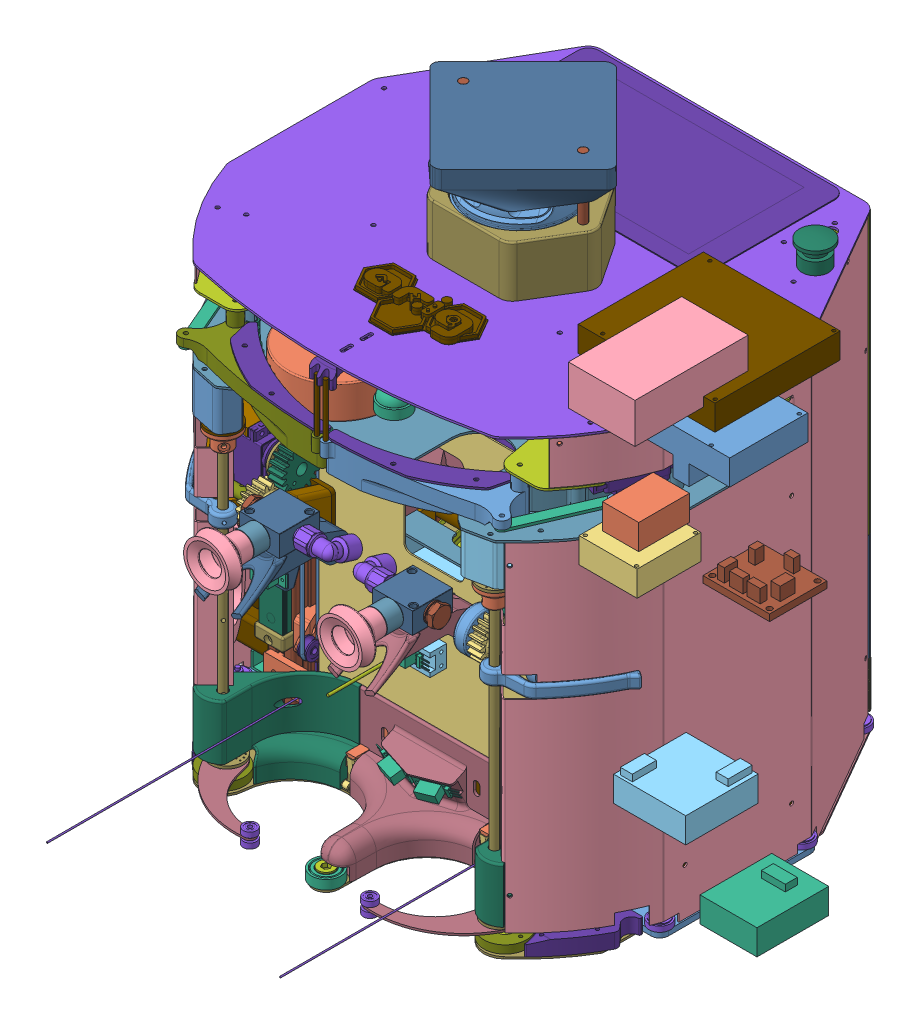
SolidWorks assembly 2019_Gros_robot, configuration Défaut. Lengths in mm.
Overall size (508.74 501.24 478.47).
582 component instances, 187 part files, 267 mates.
Components (placement in the parent):
- Robot2017_BaseRoulante-1: Robot2017_BaseRoulante [Défaut] at origin size (333 188.15 128.41)
  - Robot2015_BaseRoulante_piece01-1: Robot2015_BaseRoulante_piece01 [Défaut] at (0 7 0) size (330 4 120)
  - Robot2015_BaseRoulante_piece02-1: Robot2015_BaseRoulante_piece02 [Défaut] at (88 31 0) size (9.5 55 70)
  - Robot2015_BaseRoulante_piece02-2: Robot2015_BaseRoulante_piece02 [Défaut] at (55 31 0) x (-1 0 0) z (0 0 -1) size (9.5 55 70)
  - Robot2015_BaseRoulante_piece02-3: Robot2015_BaseRoulante_piece02 [Défaut] at (-55 31 0) size (9.5 55 70)
  - Robot2015_BaseRoulante_piece02-4: Robot2015_BaseRoulante_piece02 [Défaut] at (-88 31 0) x (-1 0 0) z (0 0 -1) size (9.5 55 70)
  - RoueMotrice-1: RoueMotrice [Défaut] at (109 -484.4772 -22.3565) x (0 -1 0) z (1 0 0) size (68.64 68.64 30)
    - Pneu-1: Pneu [Défaut] at (-515.4772 -22.3565 -15) size (64 64 30)
    - Jante-1: Jante [Défaut] at (-515.4772 -22.3565 15) x (-0.856398 -0.516316 0) z (0 0 1) size (50 50 30)
  - RoueMotrice-2: RoueMotrice [Défaut] at (-109 178.4325 494.4494) x (0 0.243951 0.969787) z (-1 0 0) size (68.64 68.64 30)
    - Pneu-1: Pneu [Défaut] at (-515.4772 -22.3565 -15) size (64 64 30)
    - Jante-1: Jante [Défaut] at (-515.4772 -22.3565 15) x (-0.856398 -0.516316 0) z (0 0 1) size (50 50 30)
  - Robot2015_BaseRoulante_piece03-1: Robot2015_BaseRoulante_piece03 [Défaut] at (117 31 0) size (67.5 12 14.69)
  - Robot2015_BaseRoulante_piece03-2: Robot2015_BaseRoulante_piece03 [Défaut] at (-117 31 0) x (-1 0 0) z (0 -0.777778 -0.62854) size (67.5 12 14.69)
  - roulement-1: roulement [Défaut] at (90 31 0) size (7 22 22)
  - roulement-2: roulement [Défaut] at (53 31 0) x (1 0 0) z (0 0.679013 0.734126) size (7 22 22)
  - roulement-3: roulement [Défaut] at (-53 31 0) x (1 0 0) z (0 0.679013 0.734126) size (7 22 22)
  - roulement-4: roulement [Défaut] at (-90 31 0) x (1 0 0) z (0 0.679013 0.734126) size (7 22 22)
  - Pignon XL037 pas5.08-1: Pignon XL037 pas5.08 [20 dents] at (67.65 31 0) x (1 0 0) z (0 -0.960015 0.27995) size (22 38 38)
  - Pignon XL037 pas5.08-2: Pignon XL037 pas5.08 [20 dents] at (67.65 149.9855 -19) x (-1 0 0) z (0 0.08811 -0.996111) size (22 38 38)
  - Robot2015_roulementAngle-1: Robot2015_roulementAngle [Défaut] at (158.5 13.75 53.5) size (16 9.5 16)
  - Robot2015_roulementAngle-2: Robot2015_roulementAngle [Défaut] at (158.5 13.75 -53.5) size (16 9.5 16)
  - Robot2015_roulementAngle-3: Robot2015_roulementAngle [Défaut] at (-158.5 13.75 53.5) size (16 9.5 16)
  - Robot2015_roulementAngle-4: Robot2015_roulementAngle [Défaut] at (-158.5 13.75 -53.5) size (16 9.5 16)
  - moteur-1: moteur [Défaut] at (48 149.9855 -19) x (0 -0.99965 -0.026437) z (1 0 0) size (42 42 188.5)
  - moteur-2: moteur [Défaut] at (-48 104.7937 -19) x (0 0.767621 0.640905) z (-1 0 0) size (42 42 188.5)
  - Pignon XL037 pas5.08-3: Pignon XL037 pas5.08 [20 dents] at (-67.65 31 0) x (-1 0 0) z (0 -0.781685 -0.623674) size (22 38 38)
  - Pignon XL037 pas5.08-4: Pignon XL037 pas5.08 [20 dents] at (-67.65 104.7937 -19) x (1 0 0) z (0 0.006752 0.999977) size (22 38 38)
  - Robot2015_profiléX20_01-1: Robot2015_profiléX20_01 [Défaut] at (-28 11 -40) x (0 0 -1) z (0 1 0) size (20 20 165)
  - Robot2015_profiléX20_01-2: Robot2015_profiléX20_01 [Défaut] at (48 11 -40) x (0 0 -1) z (0 1 0) size (20 20 165)
  - Robot2015_BaseRoulante_piece04-1: Robot2015_BaseRoulante_piece04 [Défaut] at (48 149.9855 -58) x (1 0 0) z (0 0 -1) size (3 50 44)
  - Robot2015_BaseRoulante_piece04-2: Robot2015_BaseRoulante_piece04 [Défaut] at (-51 104.7937 -58) x (1 0 0) z (0 0 -1) size (3 50 44)
  - Courroie1-5^Robot2017_BaseRoulante-1: Courroie1-5^Robot2017_BaseRoulante [Défaut] at (-67.65 104.7937 -19) x (0 0 -1) z (1 0 0) size (53.34 108.13 10) (virtual)
  - Courroie2-6^Robot2017_BaseRoulante-1: Courroie2-6^Robot2017_BaseRoulante [Défaut] at (67.65 149.9855 -19) x (0 0 1) z (-1 0 0) size (79.34 153.33 10) (virtual)
  - Robot2015_BaseRoulante_piece06-1: Robot2015_BaseRoulante_piece06 [Défaut] at (0 177.5 -61.5) size (256 20 20)
  - Igus_TK_04_09_Rail_L50-1: Igus_TK_04_09_Rail_L50 [Défaut] at (136 38.5 35) x (0 0 -1) z (1 0 0) size (9.6 50 6.3)
  - Igus_TK_04_09_coulisseau-1: Igus_TK_04_09_coulisseau [Défaut] at (136 101 35) x (0 0 -1) z (1 0 0) size (20 29 8.3)
  - Igus_TK_04_09_Rail_L50-2: Igus_TK_04_09_Rail_L50 [Défaut] at (136 38.5 -35) x (0 0 -1) z (1 0 0) size (9.6 50 6.3)
  - Igus_TK_04_09_coulisseau-2: Igus_TK_04_09_coulisseau [Défaut] at (136 101 -35) x (0 0 -1) z (1 0 0) size (20 29 8.3)
  - Igus_TK_04_09_Rail_L50-3: Igus_TK_04_09_Rail_L50 [Défaut] at (-136 38.5 35) x (0 0 1) z (-1 0 0) size (9.6 50 6.3)
  - Igus_TK_04_09_coulisseau-3: Igus_TK_04_09_coulisseau [Défaut] at (-136 101 35) x (0 0 1) z (-1 0 0) size (20 29 8.3)
  - Igus_TK_04_09_Rail_L50-4: Igus_TK_04_09_Rail_L50 [Défaut] at (-136 38.5 -35) x (0 0 1) z (-1 0 0) size (9.6 50 6.3)
  - Igus_TK_04_09_coulisseau-4: Igus_TK_04_09_coulisseau [Défaut] at (-136 101 -35) x (0 0 1) z (-1 0 0) size (20 29 8.3)
  - Kubler-05.2400.1212.1024-1: Kubler-05.2400.1212.1024 [fil a Gch] at (157 24 0) x (-1 0 0) z (0 0.34202 0.939693) size (31 88.25 62)
    - Kubler-05.2400.1212.1024-1: Kubler-05.2400.1212.1024 [Défaut] at origin size (31 36 24)
    - Kubler-rayon mini cable-1: Kubler-rayon mini cable [Défaut] at (25 -24 0) x (0 0 1) z (-1 0 0) size (52.25 52.25 4.5)
  - Kubler-05.2400.1212.1024-2: Kubler-05.2400.1212.1024 [fil a Drt] at (-157 24 0) x (1 0 0) z (0 -0.34202 -0.939693) size (31 88.25 62)
    - Kubler-05.2400.1212.1024-1: Kubler-05.2400.1212.1024 [Défaut] at origin size (31 36 24)
    - Kubler-rayon mini cable-1: Kubler-rayon mini cable [Défaut] at (25 -24 0) x (0 0 -1) z (1 0 0) size (52.25 52.25 4.5)
  - Robot2015_BaseRoulante_piece07-1: Robot2015_BaseRoulante_piece07 [Défaut] at (146 56.5 0) x (0 0 -1) z (1 0 0) size (93 50 1.5)
  - Robot2015_BaseRoulante_piece07-2: Robot2015_BaseRoulante_piece07 [Défaut] at (-146 56.5 0) x (0 0 1) z (-1 0 0) size (93 50 1.5)
  - Robot2015_BaseRoulante_piece08-1: Robot2015_BaseRoulante_piece08 [Défaut] at (51 38.5 30) size (85 55 10)
  - Robot2015_BaseRoulante_piece09-1: Robot2015_BaseRoulante_piece09 [Défaut] at (51 38.5 -30) x (1 0 0) z (0 0 -1) size (57 55 10)
  - Robot2015_BaseRoulante_piece09-2: Robot2015_BaseRoulante_piece09 [Défaut] at (-51 38.5 -30) x (-1 0 0) z (0 0 -1) size (57 55 10)
  - Robot2015_BaseRoulante_piece08-2: Robot2015_BaseRoulante_piece08 [Défaut] at (-51 38.5 30) x (-1 0 0) z (0 0 1) size (85 55 10)
  - Robot2015_BaseRoulante_piece10-1: Robot2015_BaseRoulante_piece10 [Défaut] at (155 24 0) x (-1 0 0) z (0 -0.545932 -0.837829) size (9 48 48)
  - Robot2015_BaseRoulante_piece10-2: Robot2015_BaseRoulante_piece10 [Défaut] at (-155 24 0) size (9 48 48)
  - Robot2015_BaseRoulante_piece11-1: Robot2015_BaseRoulante_piece11 [Défaut] at (79 66 0) x (0 0 -1) z (1 0 0) size (80 1.5 63)
  - Robot2015_BaseRoulante_piece11-2: Robot2015_BaseRoulante_piece11 [Défaut] at (-79 66 0) x (0 0 1) z (-1 0 0) size (80 1.5 63)
  - Robot2015_BaseRoulante_piece12-1: Robot2015_BaseRoulante_piece12 [Défaut] at (162 11 40) x (-1 0 0) z (0 0 -1) size (11.5 11.5 80)
  - Robot2015_BaseRoulante_piece12-2: Robot2015_BaseRoulante_piece12 [Défaut] at (-162 11 -40) size (11.5 11.5 80)
  - pignon renvoi 20 dents XL 2006-1: pignon renvoi 20 dents XL 2006 [Défaut] at (67.65 40 -45) x (1 0 0) z (0 0.474564 0.880221) size (9 32.34 32.34)
  - 20170402-1131-1: 20170402-1131 [Défaut] at (48 40 -45) x (0 0 -1) z (1 0 0) size (25 50 24.65)
  - 20170402-1229-1: 20170402-1229 [Défaut] at (73.15 40 -38.5) x (0 0 -1) z (1 0 0) size (25.5 30 9)
- batterieLIPO-1: batterieLIPO [Défaut] at (-65 97 -76) size (160 49 34)
- Robot2019_profiléX20_02-1: Robot2019_profiléX20_02 [Défaut] at (-110 276 40) x (0 0 1) z (0 -1 0) size (20 20 265)
- Robot2019_profiléX20_02-2: Robot2019_profiléX20_02 [Défaut] at (-110 276 -60) x (0 0 1) z (0 -1 0) size (20 20 265)
- Robot2019_profiléX20_02-3: Robot2019_profiléX20_02 [Défaut] at (130 276 40) x (0 0 1) z (0 -1 0) size (20 20 265)
- Robot2019_profiléX20_02-4: Robot2019_profiléX20_02 [Défaut] at (130 276 -60) x (0 0 1) z (0 -1 0) size (20 20 265)
- Robot2019_plaque bille porteuseAvant-1: Robot2019_plaque bille porteuseAvant [Défaut] at (0 5.5 0) size (300 1.5 120)
- Robot2019_plaque bille porteuse Arriere-1: Robot2019_plaque bille porteuse Arriere [Défaut] at (0 5.5 0) x (-1 0 0) z (0 0 -1) size (310 1.5 125)
- Robot2019_plaque du dessus-1: Robot2019_plaque du dessus [Défaut] at (0 276 0) size (330 1.5 300.96)
- APEM_A01ES_A0154B-1: APEM_A01ES_A0154B [Défaut] at (121.8383 345 -100) x (0.5 0 0.866025) z (-0.866025 0 0.5) size (24 61 24)
- bille porteuse-3: bille porteuse [Défaut] at (-111.446 0 -110) x (-0.5 0 -0.866025) z (0.866025 0 -0.5) size (49.64 21.5 47.15)
  - Robot2015_support bille porteuse-1: Robot2015_support bille porteuse [Défaut] at (0 9.5 0) size (49.64 12 45)
  - BillePorteuse-1: BillePorteuse [Défaut] at (0 7.5 0) x (0.947171 0 0.32073) z (0.32073 0 -0.947171) size (31 21.5 31)
- bille porteuse-4: bille porteuse [Défaut] at (111.446 0 -110) size (49.64 21.5 47.15)
  - Robot2015_support bille porteuse-1: Robot2015_support bille porteuse [Défaut] at (0 9.5 0) size (49.64 12 45)
  - BillePorteuse-1: BillePorteuse [Défaut] at (0 7.5 0) x (0.947171 0 0.32073) z (0.32073 0 -0.947171) size (31 21.5 31)
- pompe air 12v SFE-1: pompe air 12v SFE [Défaut] at (-20.6394 32 -38) size (38 60 92)
- rplidar-a2-1: rplidar-a2 [Défaut] at (-75 354.2861 -6.0269) x (0 0 -1) z (1 0 0) size (80.61 40.81 84.84)
- Robot2015_roulementAngle-1: Robot2015_roulementAngle [Défaut] at (100.765 9.75 -153.5) size (16 9.5 16)
- Robot2015_roulementAngle-2: Robot2015_roulementAngle [Défaut] at (-100.765 9.75 -153.5) size (16 9.5 16)
- 20180929-0119-1: 20180929-0119 [Défaut] at (0 277.5 0) x (-1 0 0) z (0 0 -1) size (291.8 157.5 260.35) (flexible)
  - Palet-1: Palet [Redium] at (-99.9974 12.7 0.7186) size (76.2 25.4 76.2)
  - Palet-2: Palet [Greenium] at (-49.3764 12.7 86.9596) size (76.2 25.4 76.2)
  - Palet-3: Palet [Redium] at (50.6211 12.7 86.241) size (76.2 25.4 76.2) (hidden)
  - Palet-4: Palet [Blueium] at (99.9974 12.7 -0.7186) x (0.648467 0 0.761243) z (-0.761243 0 0.648467) size (76.2 25.4 76.2)
  - Palet-5: Palet [Greenium] at (49.3764 12.7 -86.9596) x (0.321702 0 0.946841) z (-0.946841 0 0.321702) size (76.2 25.4 76.2)
  - Palet-6: Palet [Redium] at (-50.6211 12.7 -86.241) size (76.2 25.4 76.2) (hidden)
  - roulement-1: roulement [Défaut] at (81.9289 14.5 -48.09) x (0 -1 0) z (0.925744 0 -0.37815) size (7 22 22)
  - roulement-2: roulement [Défaut] at (-0.6827 14.5 -94.9975) x (0 -1 0) z (0.135385 0 -0.990793) size (7 22 22)
  - roulement-3: roulement [Défaut] at (-82.6116 14.5 -46.9075) x (0 -1 0) z (-0.79036 0 -0.612643) size (7 22 22)
  - roulement-4: roulement [Défaut] at (-81.9289 14.5 48.09) x (0 -1 0) z (-0.925744 0 0.37815) size (7 22 22)
  - roulement-5: roulement [Défaut] at (0.6827 14.5 94.9975) x (0 -1 0) z (-0.135385 0 0.990793) size (7 22 22)
  - roulement-6: roulement [Défaut] at (82.6116 14.5 46.9075) x (0 -1 0) z (0.79036 0 0.612643) size (7 22 22)
  - 20181010-0238-1: 20181010-0238 [Défaut] at (0 8.5 -22.5) x (0.926307 0 0.37677) z (-0.37677 0 0.926307) size (29.93 18 29.98)
  - 20181010-0239-1: 20181010-0239 [Défaut] at (0 8.5 0) x (0.853252 0 -0.521498) z (0.521498 0 0.853252) size (122.02 20.9 126.29)
  - PlaqueTounanteCarre94mm-1: PlaqueTounanteCarre94mm [Défaut] x (-0.707107 0 0.707107) z (-0.707107 0 -0.707107) size (115.6 8.5 115.6) (flexible)
    - PlaqueTounanteCarre94mm-1: PlaqueTounanteCarre94mm [Défaut] at origin size (94 8.25 94)
    - PlaqueTounanteCarre94mm-2: PlaqueTounanteCarre94mm [Défaut] at (0 8.5 0) x (-0.265754 0 -0.964041) z (-0.964041 0 0.265754) size (94 8.25 94)
  - 20190123-2151-1: 20190123-2151 [Défaut] at (0 16.5 0) x (-0.506211 0 -0.86241) z (0.86241 0 -0.506211) size (41.57 20.66 45)
  - 20190123-2208-1: 20190123-2208 [Défaut] at (81.9289 17.9 -48.09) x (-0.274765 0 -0.961511) z (-0.961511 0 0.274765) size (11.85 7.9 11.85)
  - 20190123-2208-2: 20190123-2208 [Défaut] at (-0.6827 17.9 -94.9975) x (-0.970076 0 -0.242802) z (-0.242802 0 0.970076) size (11.85 7.9 11.85)
  - 20190123-2208-3: 20190123-2208 [Défaut] at (-82.6116 17.9 -46.9075) x (-0.695311 0 0.718709) z (0.718709 0 0.695311) size (11.85 7.9 11.85)
  - 20190123-2208-4: 20190123-2208 [Défaut] at (-81.9289 17.9 48.09) x (0.274765 0 0.961511) z (0.961511 0 -0.274765) size (11.85 7.9 11.85)
  - 20190123-2208-5: 20190123-2208 [Défaut] at (0.6827 17.9 94.9975) x (0.970076 0 0.242802) z (0.242802 0 -0.970076) size (11.85 7.9 11.85)
  - 20190123-2208-6: 20190123-2208 [Défaut] at (82.6116 17.9 46.9075) x (0.695311 0 -0.718709) z (-0.718709 0 -0.695311) size (11.85 7.9 11.85)
  - 20190123-2151-2: 20190123-2151 [Défaut] at (0 16.5 0) x (-0.999974 0 0.007186) z (-0.007186 0 -0.999974) size (41.57 20.66 45)
  - 20190123-2151-3: 20190123-2151 [Défaut] at (0 16.5 0) x (-0.493764 0 0.869596) z (-0.869596 0 -0.493764) size (41.57 20.66 45)
  - 20190123-2151-4: 20190123-2151 [Défaut] at (0 16.5 0) x (0.506211 0 0.86241) z (-0.86241 0 0.506211) size (41.57 20.66 45)
  - 20190123-2151-5: 20190123-2151 [Défaut] at (0 16.5 0) x (0.999974 0 -0.007186) z (0.007186 0 0.999974) size (41.57 20.66 45)
  - 20190123-2151-6: 20190123-2151 [Défaut] at (0 16.5 0) x (0.493764 0 -0.869596) z (0.869596 0 0.493764) size (41.57 20.66 45)
  - 12v-silent-dc-motor-146rpm-encoder-desc-dime-1: 12v-silent-dc-motor-146rpm-encoder-desc-dime [Défaut] at (0 -2.5 -22.5) x (0 -1 0) z (-0.707107 0 -0.707107) size (123 36 36)
  - 20190124-0048-1: 20190124-0048 [Défaut] at (0 26.5 -22.5) size (15 43 15)
  - NBB1,5-F79-E0-1: NBB1,5-F79-E0 [Défaut] at (43 30 0) x (1 0 0) z (0 0 -1) size (21 4.7 8)
  - 20190124-0123-1: 20190124-0123 [Défaut] at (47 32 -6.05) x (0 0 1) z (-1 0 0) size (19 4 16)
- 20181001-1750-1: 20181001-1750 [Défaut] at origin size (319.23 219.5 239.4)
  - Access_HS-645_BrasRondPetitModele-2: Access_HS-645_BrasRondPetitModele [Défaut] at (94 204.5566 85.221) x (0 0.153259 -0.988186) z (0 0.988186 0.153259) size (24 5 24)
  - Palet-1: Palet [Redium] at (50 201.2365 189.2) x (1 0 0) z (0 1 0) size (76.2 25.4 76.2) (hidden)
  - Servo_HS-805-BB-1: Servo_HS-805-BB [Défaut] at (-29 228 9) x (0 0.965926 -0.258819) z (0 0.258819 0.965926) size (82 65 29.5)
  - Access_HS-805_BrasRond-1: Access_HS-805_BrasRond [Défaut] at (-89 228 9) x (0 0 -1) z (0 1 0) size (39.6 8.5 39.6)
  - HIWIN_MGW09H 1 R 200 ZF H M SS_FILE-1: HIWIN_MGW09H 1 R 200 ZF H M SS_FILE [Défaut] at (-120 68 60) size (18 200 7)
  - HIWIN_MGW09H 1 R 200 ZF H M SS_FILE_1-1: HIWIN_MGW09H 1 R 200 ZF H M SS_FILE_1 [Défaut] at (-120 164.4365 60) size (30 51.3 9.1)
  - HIWIN_MGW09H 1 R 200 ZF H M SS_FILE-2: HIWIN_MGW09H 1 R 200 ZF H M SS_FILE [Défaut] at (120 68 60) size (18 200 7)
  - HIWIN_MGW09H 1 R 200 ZF H M SS_FILE_1-2: HIWIN_MGW09H 1 R 200 ZF H M SS_FILE_1 [Défaut] at (120 164.4365 60) size (30 51.3 9.1)
  - Galet_RainureU_4x13x7-1: Galet_RainureU_4x13x7 [Défaut] at (-95.5 68 62) x (1 0 0) z (0 1 0) size (7 13 13)
  - Galet_RainureU_4x13x7-2: Galet_RainureU_4x13x7 [Défaut] at (-95.5 188 50) x (1 0 0) z (0 1 0) size (7 13 13)
  - 20190123-2357-1: 20190123-2357 [Défaut] at (-98 228 9) x (1 0 0) z (0 0 -1) size (7 93 93)
  - Galet_RainureU_4x13x7-5: Galet_RainureU_4x13x7 [Défaut] at (-95.5 248 62) x (1 0 0) z (0 1 0) size (7 13 13)
  - 20190124-0203-1: 20190124-0203 [Défaut] at (-95.5 68 68) x (0 0 1) z (-1 0 0) size (104.52 211.5 2.55)
  - Servo_HS-805-BB-3: Servo_HS-805-BB [Défaut] at (29 228 9) x (0 0.965926 -0.258819) z (0 -0.258819 -0.965926) size (82 65 29.5)
  - SymétrieAccess_HS-805_BrasRond-3: SymétrieAccess_HS-805_BrasRond [Défaut] at (89 228 9) x (0 0 -1) z (0 -1 0) size (39.6 8.5 39.6)
  - 20190123-2357-3: 20190123-2357 [Défaut] at (98 228 9) x (-1 0 0) z (0 0 1) size (7 93 93)
  - Symétrie20190124-0203-2: Symétrie20190124-0203 [Défaut] at (95.5 68 68) x (0 0 1) z (-1 0 0) size (104.5 211.5 2.5)
  - Galet_RainureU_4x13x7-7: Galet_RainureU_4x13x7 [Défaut] at (95.5 248 62) x (-1 0 0) z (0 -1 0) size (7 13 13)
  - Galet_RainureU_4x13x7-8: Galet_RainureU_4x13x7 [Défaut] at (95.5 188 50) x (-1 0 0) z (0 -1 0) size (7 13 13)
  - Galet_RainureU_4x13x7-9: Galet_RainureU_4x13x7 [Défaut] at (95.5 68 62) x (-1 0 0) z (0 -1 0) size (7 13 13)
  - Ventouse_D33-1: Ventouse_D33 [Défaut] at (50 206.2365 176.5) x (1 0 0) z (0 1 0) size (36.31 27 36.31)
  - 20170416-2304-1: 20170416-2304 [Défaut] at (54 176.4365 124) size (30.6 16 70.4)
    - SupportCapteurPololu-1: SupportCapteurPololu [Défaut] at origin size (30 16 12.5) (hidden)
    - pololu gp2y0d805-1: pololu gp2y0d805 [Défaut] at (-14.5 -4.5 10.8) size (30.1 9 11.8)
    - faisceau pololu gp2y0d-1: faisceau pololu gp2y0d [5cm] at (-3.9 0 20.4) size (2 2 50) (hidden)
  - Legris_EQUERRE-OSCILLANTE_3159_06_10-1: Legris_EQUERRE-OSCILLANTE_3159_06_10 [Défaut] at (40 206.2365 130.5) x (0 -0.296934 -0.954898) z (0 0.954898 -0.296934) size (28 34.3 15.01)
  - Legris_DouilleAnnelee_0934_10_10-1: Legris_DouilleAnnelee_0934_10_10 [Défaut] at (50 206.2365 151) x (-0.990503 0.137493 0) z (0.137493 0.990503 0) size (15.24 32.5 12)
  - Legris_NourriceCroix_3312_00_10-1: Legris_NourriceCroix_3312_00_10 [Défaut] at (50 198.2365 130.5) x (1 0 0) z (0 1 0) size (30 30 16)
  - Legris_Bouchon_0220_10_00-1: Legris_Bouchon_0220_10_00 [Défaut] at (67.975 206.2365 130.5) x (-1 0 0) z (0 -1 0) size (12.5 14 16.17)
  - 20181010-0238-2: 20181010-0238 [Défaut] at (78 184.2365 103) x (0 0.752597 -0.658481) z (0 -0.658481 -0.752597) size (29.93 18 29.98)
  - roulement_D8-D16-ep4-2: roulement_D8-D16-ep4 [Défaut] at (121.5 184.2365 103) x (1 0 0) z (0 -0.7977 0.603055) size (4 16 16)
  - 20190206-2329-1: 20190206-2329 [Défaut] at (50 206.2365 176.5) size (36.88 28.38 83.9)
  - 20190207-0044-1: 20190207-0044 [Défaut] at (50 206.2365 158.5) x (0.792778 -0.60951 0) z (0 0 -1) size (18 18 13)
  - 20181010-0240-1: 20181010-0240 [Défaut] at (78.5 204.5566 85.221) x (0 0.752597 -0.658481) z (0 -0.658481 -0.752597) size (29.93 11 29.98)
  - 20190207-0111-1: 20190207-0111 [Défaut] at (33.5 184.2365 103) x (0 -0.34202 -0.939693) z (-1 0 0) size (8 8 90)
  - roulement-1: roulement [Défaut] at (70 184.2365 103) size (7 22 22)
  - Servo_HS-645-MG_2-1: Servo_HS-645-MG_2 [Défaut] at (134.238 174.3306 75.442) x (0 0 1) z (0 -1 0) size (19.56 43.24 53.34)
  - 20190208-1431-1: 20190208-1431 [Défaut] at (66.5 164.2365 72) size (75 57 3)
  - 20190208-1506-1: 20190208-1506 [Défaut] at (109 221.2365 75) x (1 0 0) z (0 -1 0) size (76.02 43 57.11)
  - 20190209-0034-1: 20190209-0034 [Défaut] at (-110 68 50) x (0 0 1) z (1 0 0) size (24.5 25 12.5)
  - 20190209-0034-2: 20190209-0034 [Défaut] at (-110 248 50) x (0 0 1) z (1 0 0) size (24.5 25 12.5)
  - 20190209-0206-1: 20190209-0206 [Défaut] at (-110 200.5 50) x (0 0 -1) z (1 0 0) size (16 25 12.5)
  - 20190209-0206-2: 20190209-0206 [Défaut] at (110 200.5 50) x (0 0 1) z (-1 0 0) size (16 25 12.5)
  - 20190209-0034-3: 20190209-0034 [Défaut] at (110 248 50) x (0 0 1) z (-1 0 0) size (24.5 25 12.5)
  - 20190209-0034-4: 20190209-0034 [Défaut] at (110 68 50) x (0 0 1) z (-1 0 0) size (24.5 25 12.5)
  - 20190211-2116-1: 20190211-2116 [Défaut] at (148.047 126.5 67.5372) x (0.819152 0 0.573576) z (-0.573576 0 0.819152) size (12 78.68 50)
  - Igus_ChainePorteCable_ExtremiteA_modif2019-1: Igus_ChainePorteCable_ExtremiteA_modif2019 [Défaut] at (150.9141 126.5 69.5447) x (0 1 0) z (-0.573576 0 0.819152) size (26 36.15 16.39)
  - Igus_ChainePorteCable_ExtremiteB_modif2019-1: Igus_ChainePorteCable_ExtremiteB_modif2019 [Défaut] at (155.7489 239.4042 62.6133) x (0.099601 0.984808 -0.142244) z (-0.564863 0.173648 0.806707) size (25.74 12 18.61)
  - 20190212-2242-1: 20190212-2242 [Défaut] at (93.5 179.2365 72) size (8 24 3.9)
  - 20190212-2242-2: 20190212-2242 [Défaut] at (93.5 179.2365 64.2) x (1 0 0) z (0 0 -1) size (8 24 3.9)
  - 20190328-0013-1: 20190328-0013 [Défaut] at (73.5 184.2365 103) x (0 -0.835831 -0.548987) z (0 -0.548987 0.835831) size (14 4.5 14)
  - 20190208-1431-2: 20190208-1431 [Défaut] at (-66.5 164.2365 75) x (-1 0 0) z (0 0 -1) size (75 57 3)
  - Symétrie20190208-1506-2: Symétrie20190208-1506 [Défaut] at (-109 221.2365 75) x (-1 0 0) z (0 1 0) size (76.02 43 57.11)
  - Servo_HS-645-MG_2-2: Servo_HS-645-MG_2 [Défaut] at (-134.238 174.3306 95) x (0 0 -1) z (0 -1 0) size (19.56 43.24 53.34)
  - Access_HS-645_BrasRondPetitModele-3: Access_HS-645_BrasRondPetitModele [Défaut] at (-89 204.5566 85.221) x (0 -0.153259 0.988186) z (0 -0.988186 -0.153259) size (24 5 24)
  - 20181010-0240-2: 20181010-0240 [Défaut] at (-89.5 204.5566 85.221) x (0 0.752597 -0.658481) z (0 -0.658481 -0.752597) size (29.93 11 29.98)
  - 20181010-0238-3: 20181010-0238 [Défaut] at (-96 184.2365 103) x (0 0.752597 -0.658481) z (0 -0.658481 -0.752597) size (29.93 18 29.98)
  - 20190328-0013-2: 20190328-0013 [Défaut] at (-73.5 184.2365 103) x (0 -0.835831 -0.548987) z (0 0.548987 -0.835831) size (14 4.5 14)
  - 20190207-0111-2: 20190207-0111 [Défaut] at (-123.5 184.2365 103) x (0 -0.34202 -0.939693) z (-1 0 0) size (8 8 90)
  - Symétrie20190206-2329-2: Symétrie20190206-2329 [Défaut] at (-50 206.2365 176.5) x (-1 0 0) z (0 0 -1) size (36.88 28.38 83.9)
  - roulement_D8-D16-ep4-3: roulement_D8-D16-ep4 [Défaut] at (-121.5 184.2365 103) x (-1 0 0) z (0 0.7977 -0.603055) size (4 16 16)
  - roulement-2: roulement [Défaut] at (-70 184.2365 103) x (-1 0 0) z (0 0 -1) size (7 22 22)
  - 20170416-2304-2: 20170416-2304 [Défaut] at (-54 176.4365 124) x (-1 0 0) z (0 0 1) size (30.6 16 70.4)
    - SupportCapteurPololu-1: SupportCapteurPololu [Défaut] at origin size (30 16 12.5) (hidden)
    - pololu gp2y0d805-1: pololu gp2y0d805 [Défaut] at (-14.5 -4.5 10.8) size (30.1 9 11.8)
    - faisceau pololu gp2y0d-1: faisceau pololu gp2y0d [5cm] at (-3.9 0 20.4) size (2 2 50) (hidden)
  - Legris_NourriceCroix_3312_00_10-2: Legris_NourriceCroix_3312_00_10 [Défaut] at (-50 214.2365 130.5) x (-1 0 0) z (0 -1 0) size (30 30 16)
  - Legris_Bouchon_0220_10_00-2: Legris_Bouchon_0220_10_00 [Défaut] at (-67.975 206.2365 130.5) x (1 0 0) z (0 1 0) size (12.5 14 16.17)
  - SymétrieIgus_ChainePorteCable_ExtremiteA_modif2019-2: SymétrieIgus_ChainePorteCable_ExtremiteA_modif2019 [Défaut] at (-150.9141 126.5 69.5447) x (0 1 0) z (-0.573576 0 -0.819152) size (26 36.15 16.39)
  - 20190211-2116-2: 20190211-2116 [Défaut] at (-148.047 126.5 67.5372) x (0.819152 0 -0.573576) z (0.573576 0 0.819152) size (12 78.68 50)
  - Igus_ChainePorteCable_ExtremiteB_modif2019-2: Igus_ChainePorteCable_ExtremiteB_modif2019 [Défaut] at (-150.0148 239.4042 58.5983) x (-0.099601 0.984808 -0.142244) z (0.564863 0.173648 0.806707) size (25.74 12 18.61)
  - 20190207-0044-2: 20190207-0044 [Défaut] at (-50 206.2365 158.5) x (0.792778 0.60951 0) z (0 0 -1) size (18 18 13)
  - Ventouse_D33-2: Ventouse_D33 [Défaut] at (-50 206.2365 176.5) x (-1 0 0) z (0 -1 0) size (36.31 27 36.31)
  - Legris_DouilleAnnelee_0934_10_10-2: Legris_DouilleAnnelee_0934_10_10 [Défaut] at (-50 206.2365 151) x (0.990503 0.137493 0) z (0.137493 -0.990503 0) size (15.24 32.5 12)
  - Legris_EQUERRE-OSCILLANTE_3159_06_10-2: Legris_EQUERRE-OSCILLANTE_3159_06_10 [Défaut] at (-40 206.2365 130.5) x (0 -0.296934 -0.954898) z (0 -0.954898 0.296934) size (28 34.3 15.01)
  - 20190409-2355-1: 20190409-2355 [Défaut] at (120 61 60) size (22 10 10.2)
  - 20190409-2355-2: 20190409-2355 [Défaut] at (120 275 60) x (-1 0 0) z (0 0 1) size (22 10 10.2)
  - 20190409-2355-3: 20190409-2355 [Défaut] at (-120 275 60) x (-1 0 0) z (0 0 1) size (22 10 10.2)
  - 20190409-2355-4: 20190409-2355 [Défaut] at (-120 61 60) size (22 10 10.2)
- 20181001-2148-1: 20181001-2148 [Défaut] at (-50 7 120) size (106 62 83)
- 20181002-0030-1: 20181002-0030 [Défaut] at (0 277.5 0) x (0.725374 0 0.688355) z (-0.688355 0 0.725374) size (312.09 32 306.03)
  - 20181002-0031-1: 20181002-0031 [Défaut] at origin size (146.08 16 151.84)
  - BagueRivetAIRBUS-1: BagueRivetAIRBUS [Défaut] at (141.5 15.8 0) x (0.352131 0 0.935951) z (0 1 0) size (6.8 6.8 5.6)
  - BagueRivetAIRBUS-2: BagueRivetAIRBUS [Défaut] at (141.3061 15.8 -7.4055) x (0.400633 0 0.916239) z (0 1 0) size (6.8 6.8 5.6)
  - BagueRivetAIRBUS-3: BagueRivetAIRBUS [Défaut] at (140.7248 15.8 -14.7908) x (0.448036 0 0.894016) z (0 1 0) size (6.8 6.8 5.6)
  - BagueRivetAIRBUS-4: BagueRivetAIRBUS [Défaut] at (139.7579 15.8 -22.1355) x (0.494211 0 0.869342) z (0 1 0) size (6.8 6.8 5.6)
  - BagueRivetAIRBUS-5: BagueRivetAIRBUS [Défaut] at (138.4079 15.8 -29.4195) x (0.539032 0 0.842286) z (0 1 0) size (6.8 6.8 5.6)
  - BagueRivetAIRBUS-6: BagueRivetAIRBUS [Défaut] at (136.6785 15.8 -36.6229) x (0.582375 0 0.812921) z (0 1 0) size (6.8 6.8 5.6)
  - BagueRivetAIRBUS-7: BagueRivetAIRBUS [Défaut] at (134.5745 15.8 -43.7259) x (0.624122 0 0.781327) z (0 1 0) size (6.8 6.8 5.6)
  - BagueRivetAIRBUS-8: BagueRivetAIRBUS [Défaut] at (132.1016 15.8 -50.7091) x (0.664158 0 0.747593) z (0 1 0) size (6.8 6.8 5.6)
  - BagueRivetAIRBUS-9: BagueRivetAIRBUS [Défaut] at (129.2667 15.8 -57.5532) x (0.702373 0 0.711809) z (0 1 0) size (6.8 6.8 5.6)
  - BagueRivetAIRBUS-10: BagueRivetAIRBUS [Défaut] at (126.0774 15.8 -64.2397) x (0.738664 0 0.674074) z (0 1 0) size (6.8 6.8 5.6)
  - BagueRivetAIRBUS-11: BagueRivetAIRBUS [Défaut] at (122.5426 15.8 -70.75) x (0.77293 0 0.634491) z (0 1 0) size (6.8 6.8 5.6)
  - BagueRivetAIRBUS-12: BagueRivetAIRBUS [Défaut] at (118.6719 15.8 -77.0664) x (0.805077 0 0.59317) z (0 1 0) size (6.8 6.8 5.6)
  - BagueRivetAIRBUS-13: BagueRivetAIRBUS [Défaut] at (114.4759 15.8 -83.1716) x (0.835018 0 0.550222) z (0 1 0) size (6.8 6.8 5.6)
  - BagueRivetAIRBUS-14: BagueRivetAIRBUS [Défaut] at (109.9662 15.8 -89.0488) x (0.86267 0 0.505767) z (0 1 0) size (6.8 6.8 5.6)
  - BagueRivetAIRBUS-15: BagueRivetAIRBUS [Défaut] at (105.155 15.8 -94.682) x (0.887958 0 0.459925) z (0 1 0) size (6.8 6.8 5.6)
  - BagueRivetAIRBUS-16: BagueRivetAIRBUS [Défaut] at (100.0556 15.8 -100.0556) x (0.910812 0 0.412822) z (0 1 0) size (6.8 6.8 5.6)
  - BagueRivetAIRBUS-17: BagueRivetAIRBUS [Défaut] at (94.682 15.8 -105.155) x (0.931169 0 0.364589) z (0 1 0) size (6.8 6.8 5.6)
  - BagueRivetAIRBUS-18: BagueRivetAIRBUS [Défaut] at (89.0488 15.8 -109.9662) x (0.948974 0 0.315355) z (0 1 0) size (6.8 6.8 5.6)
  - BagueRivetAIRBUS-19: BagueRivetAIRBUS [Défaut] at (83.1716 15.8 -114.4759) x (0.964178 0 0.265258) z (0 1 0) size (6.8 6.8 5.6)
  - BagueRivetAIRBUS-20: BagueRivetAIRBUS [Défaut] at (77.0664 15.8 -118.6719) x (0.976739 0 0.214433) z (0 1 0) size (6.8 6.8 5.6)
  - BagueRivetAIRBUS-21: BagueRivetAIRBUS [Défaut] at (70.75 15.8 -122.5426) x (0.986623 0 0.163021) z (0 1 0) size (6.8 6.8 5.6)
  - BagueRivetAIRBUS-22: BagueRivetAIRBUS [Défaut] at (64.2397 15.8 -126.0774) x (0.993802 0 0.111161) z (0 1 0) size (6.8 6.8 5.6)
  - BagueRivetAIRBUS-23: BagueRivetAIRBUS [Défaut] at (57.5532 15.8 -129.2667) x (0.998258 0 0.058997) z (0 1 0) size (6.8 6.8 5.6)
  - BagueRivetAIRBUS-24: BagueRivetAIRBUS [Défaut] at (50.7091 15.8 -132.1016) x (0.999978 0 0.006672) z (0 1 0) size (6.8 6.8 5.6)
  - BagueRivetAIRBUS-25: BagueRivetAIRBUS [Défaut] at (43.7259 15.8 -134.5745) x (0.998956 0 -0.045672) z (0 1 0) size (6.8 6.8 5.6)
  - BagueRivetAIRBUS-26: BagueRivetAIRBUS [Défaut] at (36.6229 15.8 -136.6785) x (0.995197 0 -0.097891) z (0 1 0) size (6.8 6.8 5.6)
  - BagueRivetAIRBUS-27: BagueRivetAIRBUS [Défaut] at (29.4195 15.8 -138.4079) x (0.98871 0 -0.149841) z (0 1 0) size (6.8 6.8 5.6)
  - BagueRivetAIRBUS-28: BagueRivetAIRBUS [Défaut] at (22.1355 15.8 -139.7579) x (0.979513 0 -0.201381) z (0 1 0) size (6.8 6.8 5.6)
  - BagueRivetAIRBUS-29: BagueRivetAIRBUS [Défaut] at (14.7908 15.8 -140.7248) x (0.967631 0 -0.252369) z (0 1 0) size (6.8 6.8 5.6)
  - BagueRivetAIRBUS-30: BagueRivetAIRBUS [Défaut] at (7.4055 15.8 -141.3061) x (0.953097 0 -0.302665) z (0 1 0) size (6.8 6.8 5.6)
  - 20181002-0031-2: 20181002-0031 [Défaut] at (0 32 0) x (0.052336 0 -0.99863) z (-0.99863 0 -0.052336) size (146.08 16 151.84)
  - 20181002-0031-3: 20181002-0031 [Défaut] x (0 0 -1) z (1 0 0) size (146.08 16 151.84)
  - 20181002-0031-4: 20181002-0031 [Défaut] x (-1 0 0) z (0 0 -1) size (146.08 16 151.84)
  - BagueRivetAIRBUS-91: BagueRivetAIRBUS [Défaut] at (0 15.8 -141.5) x (0.935951 0 -0.352131) z (0 1 0) size (6.8 6.8 5.6)
  - BagueRivetAIRBUS-92: BagueRivetAIRBUS [Défaut] at (-141.5 15.8 0) x (-0.352131 0 -0.935951) z (0 1 0) size (6.8 6.8 5.6)
  - BagueRivetAIRBUS-93: BagueRivetAIRBUS [Défaut] at (-7.4055 15.8 -141.3061) x (0.916239 0 -0.400633) z (0 1 0) size (6.8 6.8 5.6)
  - BagueRivetAIRBUS-94: BagueRivetAIRBUS [Défaut] at (-141.3061 15.8 7.4055) x (-0.400633 0 -0.916239) z (0 1 0) size (6.8 6.8 5.6)
  - BagueRivetAIRBUS-95: BagueRivetAIRBUS [Défaut] at (-29.4195 15.8 -138.4079) x (0.842286 0 -0.539032) z (0 1 0) size (6.8 6.8 5.6)
  - BagueRivetAIRBUS-96: BagueRivetAIRBUS [Défaut] at (-138.4079 15.8 29.4195) x (-0.539032 0 -0.842286) z (0 1 0) size (6.8 6.8 5.6)
  - BagueRivetAIRBUS-97: BagueRivetAIRBUS [Défaut] at (-22.1355 15.8 -139.7579) x (0.869342 0 -0.494211) z (0 1 0) size (6.8 6.8 5.6)
  - BagueRivetAIRBUS-98: BagueRivetAIRBUS [Défaut] at (-139.7579 15.8 22.1355) x (-0.494211 0 -0.869342) z (0 1 0) size (6.8 6.8 5.6)
  - BagueRivetAIRBUS-99: BagueRivetAIRBUS [Défaut] at (-36.6229 15.8 -136.6785) x (0.812921 0 -0.582375) z (0 1 0) size (6.8 6.8 5.6)
  - BagueRivetAIRBUS-100: BagueRivetAIRBUS [Défaut] at (-136.6785 15.8 36.6229) x (-0.582375 0 -0.812921) z (0 1 0) size (6.8 6.8 5.6)
  - BagueRivetAIRBUS-101: BagueRivetAIRBUS [Défaut] at (-43.7259 15.8 -134.5745) x (0.781327 0 -0.624122) z (0 1 0) size (6.8 6.8 5.6)
  - BagueRivetAIRBUS-102: BagueRivetAIRBUS [Défaut] at (-134.5745 15.8 43.7259) x (-0.624122 0 -0.781327) z (0 1 0) size (6.8 6.8 5.6)
  - BagueRivetAIRBUS-103: BagueRivetAIRBUS [Défaut] at (-14.7908 15.8 -140.7248) x (0.894016 0 -0.448036) z (0 1 0) size (6.8 6.8 5.6)
  - BagueRivetAIRBUS-104: BagueRivetAIRBUS [Défaut] at (-140.7248 15.8 14.7908) x (-0.448036 0 -0.894016) z (0 1 0) size (6.8 6.8 5.6)
  - BagueRivetAIRBUS-105: BagueRivetAIRBUS [Défaut] at (-50.7091 15.8 -132.1016) x (0.747593 0 -0.664158) z (0 1 0) size (6.8 6.8 5.6)
  - BagueRivetAIRBUS-106: BagueRivetAIRBUS [Défaut] at (-132.1016 15.8 50.7091) x (-0.664158 0 -0.747593) z (0 1 0) size (6.8 6.8 5.6)
  - BagueRivetAIRBUS-107: BagueRivetAIRBUS [Défaut] at (-64.2397 15.8 -126.0774) x (0.674074 0 -0.738664) z (0 1 0) size (6.8 6.8 5.6)
  - BagueRivetAIRBUS-108: BagueRivetAIRBUS [Défaut] at (-126.0774 15.8 64.2397) x (-0.738664 0 -0.674074) z (0 1 0) size (6.8 6.8 5.6)
  - BagueRivetAIRBUS-109: BagueRivetAIRBUS [Défaut] at (-70.75 15.8 -122.5426) x (0.634491 0 -0.77293) z (0 1 0) size (6.8 6.8 5.6)
  - BagueRivetAIRBUS-110: BagueRivetAIRBUS [Défaut] at (-122.5426 15.8 70.75) x (-0.77293 0 -0.634491) z (0 1 0) size (6.8 6.8 5.6)
  - BagueRivetAIRBUS-111: BagueRivetAIRBUS [Défaut] at (-100.0556 15.8 -100.0556) x (0.412822 0 -0.910812) z (0 1 0) size (6.8 6.8 5.6)
  - BagueRivetAIRBUS-112: BagueRivetAIRBUS [Défaut] at (-100.0556 15.8 100.0556) x (-0.910812 0 -0.412822) z (0 1 0) size (6.8 6.8 5.6)
  - BagueRivetAIRBUS-113: BagueRivetAIRBUS [Défaut] at (-122.5426 15.8 -70.75) x (0.163021 0 -0.986623) z (0 1 0) size (6.8 6.8 5.6)
  - BagueRivetAIRBUS-114: BagueRivetAIRBUS [Défaut] at (-70.75 15.8 122.5426) x (-0.986623 0 -0.163021) z (0 1 0) size (6.8 6.8 5.6)
  - BagueRivetAIRBUS-115: BagueRivetAIRBUS [Défaut] at (-94.682 15.8 -105.155) x (0.459925 0 -0.887958) z (0 1 0) size (6.8 6.8 5.6)
  - BagueRivetAIRBUS-116: BagueRivetAIRBUS [Défaut] at (-105.155 15.8 94.682) x (-0.887958 0 -0.459925) z (0 1 0) size (6.8 6.8 5.6)
  - BagueRivetAIRBUS-117: BagueRivetAIRBUS [Défaut] at (-129.2667 15.8 -57.5532) x (0.058997 0 -0.998258) z (0 1 0) size (6.8 6.8 5.6)
  - BagueRivetAIRBUS-118: BagueRivetAIRBUS [Défaut] at (-57.5532 15.8 129.2667) x (-0.998258 0 -0.058997) z (0 1 0) size (6.8 6.8 5.6)
  - BagueRivetAIRBUS-119: BagueRivetAIRBUS [Défaut] at (-136.6785 15.8 -36.6229) x (-0.097891 0 -0.995197) z (0 1 0) size (6.8 6.8 5.6)
  - BagueRivetAIRBUS-120: BagueRivetAIRBUS [Défaut] at (-36.6229 15.8 136.6785) x (-0.995197 0 0.097891) z (0 1 0) size (6.8 6.8 5.6)
  - BagueRivetAIRBUS-121: BagueRivetAIRBUS [Défaut] at (-141.3061 15.8 -7.4055) x (-0.302665 0 -0.953097) z (0 1 0) size (6.8 6.8 5.6)
  - BagueRivetAIRBUS-122: BagueRivetAIRBUS [Défaut] at (-7.4055 15.8 141.3061) x (-0.953097 0 0.302665) z (0 1 0) size (6.8 6.8 5.6)
  - BagueRivetAIRBUS-123: BagueRivetAIRBUS [Défaut] at (-77.0664 15.8 -118.6719) x (0.59317 0 -0.805077) z (0 1 0) size (6.8 6.8 5.6)
  - BagueRivetAIRBUS-124: BagueRivetAIRBUS [Défaut] at (-118.6719 15.8 77.0664) x (-0.805077 0 -0.59317) z (0 1 0) size (6.8 6.8 5.6)
  - BagueRivetAIRBUS-125: BagueRivetAIRBUS [Défaut] at (-118.6719 15.8 -77.0664) x (0.214433 0 -0.976739) z (0 1 0) size (6.8 6.8 5.6)
  - BagueRivetAIRBUS-126: BagueRivetAIRBUS [Défaut] at (-77.0664 15.8 118.6719) x (-0.976739 0 -0.214433) z (0 1 0) size (6.8 6.8 5.6)
  - BagueRivetAIRBUS-127: BagueRivetAIRBUS [Défaut] at (-139.7579 15.8 -22.1355) x (-0.201381 0 -0.979513) z (0 1 0) size (6.8 6.8 5.6)
  - BagueRivetAIRBUS-128: BagueRivetAIRBUS [Défaut] at (-22.1355 15.8 139.7579) x (-0.979513 0 0.201381) z (0 1 0) size (6.8 6.8 5.6)
  - BagueRivetAIRBUS-129: BagueRivetAIRBUS [Défaut] at (-57.5532 15.8 -129.2667) x (0.711809 0 -0.702373) z (0 1 0) size (6.8 6.8 5.6)
  - BagueRivetAIRBUS-130: BagueRivetAIRBUS [Défaut] at (-129.2667 15.8 57.5532) x (-0.702373 0 -0.711809) z (0 1 0) size (6.8 6.8 5.6)
  - BagueRivetAIRBUS-131: BagueRivetAIRBUS [Défaut] at (-105.155 15.8 -94.682) x (0.364589 0 -0.931169) z (0 1 0) size (6.8 6.8 5.6)
  - BagueRivetAIRBUS-132: BagueRivetAIRBUS [Défaut] at (-94.682 15.8 105.155) x (-0.931169 0 -0.364589) z (0 1 0) size (6.8 6.8 5.6)
  - BagueRivetAIRBUS-133: BagueRivetAIRBUS [Défaut] at (-126.0774 15.8 -64.2397) x (0.111161 0 -0.993802) z (0 1 0) size (6.8 6.8 5.6)
  - BagueRivetAIRBUS-134: BagueRivetAIRBUS [Défaut] at (-64.2397 15.8 126.0774) x (-0.993802 0 -0.111161) z (0 1 0) size (6.8 6.8 5.6)
  - BagueRivetAIRBUS-135: BagueRivetAIRBUS [Défaut] at (-109.9662 15.8 -89.0488) x (0.315355 0 -0.948974) z (0 1 0) size (6.8 6.8 5.6)
  - BagueRivetAIRBUS-136: BagueRivetAIRBUS [Défaut] at (-89.0488 15.8 109.9662) x (-0.948974 0 -0.315355) z (0 1 0) size (6.8 6.8 5.6)
  - BagueRivetAIRBUS-137: BagueRivetAIRBUS [Défaut] at (-132.1016 15.8 -50.7091) x (0.006672 0 -0.999978) z (0 1 0) size (6.8 6.8 5.6)
  - BagueRivetAIRBUS-138: BagueRivetAIRBUS [Défaut] at (-50.7091 15.8 132.1016) x (-0.999978 0 -0.006672) z (0 1 0) size (6.8 6.8 5.6)
  - BagueRivetAIRBUS-139: BagueRivetAIRBUS [Défaut] at (-138.4079 15.8 -29.4195) x (-0.149841 0 -0.98871) z (0 1 0) size (6.8 6.8 5.6)
  - BagueRivetAIRBUS-140: BagueRivetAIRBUS [Défaut] at (-29.4195 15.8 138.4079) x (-0.98871 0 0.149841) z (0 1 0) size (6.8 6.8 5.6)
  - BagueRivetAIRBUS-141: BagueRivetAIRBUS [Défaut] at (-134.5745 15.8 -43.7259) x (-0.045672 0 -0.998956) z (0 1 0) size (6.8 6.8 5.6)
  - BagueRivetAIRBUS-142: BagueRivetAIRBUS [Défaut] at (-43.7259 15.8 134.5745) x (-0.998956 0 0.045672) z (0 1 0) size (6.8 6.8 5.6)
  - BagueRivetAIRBUS-143: BagueRivetAIRBUS [Défaut] at (-140.7248 15.8 -14.7908) x (-0.252369 0 -0.967631) z (0 1 0) size (6.8 6.8 5.6)
  - BagueRivetAIRBUS-144: BagueRivetAIRBUS [Défaut] at (-14.7908 15.8 140.7248) x (-0.967631 0 0.252369) z (0 1 0) size (6.8 6.8 5.6)
  - BagueRivetAIRBUS-145: BagueRivetAIRBUS [Défaut] at (-83.1716 15.8 -114.4759) x (0.550222 0 -0.835018) z (0 1 0) size (6.8 6.8 5.6)
  - BagueRivetAIRBUS-146: BagueRivetAIRBUS [Défaut] at (-114.4759 15.8 83.1716) x (-0.835018 0 -0.550222) z (0 1 0) size (6.8 6.8 5.6)
  - BagueRivetAIRBUS-147: BagueRivetAIRBUS [Défaut] at (-89.0488 15.8 -109.9662) x (0.505767 0 -0.86267) z (0 1 0) size (6.8 6.8 5.6)
  - BagueRivetAIRBUS-148: BagueRivetAIRBUS [Défaut] at (-109.9662 15.8 89.0488) x (-0.86267 0 -0.505767) z (0 1 0) size (6.8 6.8 5.6)
  - BagueRivetAIRBUS-149: BagueRivetAIRBUS [Défaut] at (-114.4759 15.8 -83.1716) x (0.265258 0 -0.964178) z (0 1 0) size (6.8 6.8 5.6)
  - BagueRivetAIRBUS-150: BagueRivetAIRBUS [Défaut] at (-83.1716 15.8 114.4759) x (-0.964178 0 -0.265258) z (0 1 0) size (6.8 6.8 5.6)
  - 20181002-0031-5: 20181002-0031 [Défaut] at (0 32 0) x (-0.99863 0 -0.052336) z (-0.052336 0 0.99863) size (146.08 16 151.84)
  - 20181002-0031-6: 20181002-0031 [Défaut] at (0 32 0) x (-0.052336 0 0.99863) z (0.99863 0 0.052336) size (146.08 16 151.84)
- 20181002-0216-1: 20181002-0216 [Défaut] at (0 277.5 0) x (-0.688355 0 0.725374) z (-0.725374 0 -0.688355) size (81.93 62 112.21)
  - 20181002-0217-1: 20181002-0217 [Défaut] at origin size (81.17 33 112.21)
  - BagueRivetAIRBUS-1: BagueRivetAIRBUS [Défaut] at (141.5 15.8 0) x (0.352131 0 0.935951) z (0 1 0) size (6.8 6.8 5.6)
  - BagueRivetAIRBUS-2: BagueRivetAIRBUS [Défaut] at (141.3061 15.8 -7.4055) x (0.400633 0 0.916239) z (0 1 0) size (6.8 6.8 5.6)
  - BagueRivetAIRBUS-3: BagueRivetAIRBUS [Défaut] at (140.7248 15.8 -14.7908) x (0.448036 0 0.894016) z (0 1 0) size (6.8 6.8 5.6)
  - BagueRivetAIRBUS-4: BagueRivetAIRBUS [Défaut] at (139.7579 15.8 -22.1355) x (0.494211 0 0.869342) z (0 1 0) size (6.8 6.8 5.6)
  - BagueRivetAIRBUS-5: BagueRivetAIRBUS [Défaut] at (138.4079 15.8 -29.4195) x (0.539032 0 0.842286) z (0 1 0) size (6.8 6.8 5.6)
  - BagueRivetAIRBUS-6: BagueRivetAIRBUS [Défaut] at (136.6785 15.8 -36.6229) x (0.582375 0 0.812921) z (0 1 0) size (6.8 6.8 5.6)
  - BagueRivetAIRBUS-7: BagueRivetAIRBUS [Défaut] at (134.5745 15.8 -43.7259) x (0.624122 0 0.781327) z (0 1 0) size (6.8 6.8 5.6)
  - BagueRivetAIRBUS-8: BagueRivetAIRBUS [Défaut] at (132.1016 15.8 -50.7091) x (0.664158 0 0.747593) z (0 1 0) size (6.8 6.8 5.6)
  - BagueRivetAIRBUS-9: BagueRivetAIRBUS [Défaut] at (129.2667 15.8 -57.5532) x (0.702373 0 0.711809) z (0 1 0) size (6.8 6.8 5.6)
  - BagueRivetAIRBUS-10: BagueRivetAIRBUS [Défaut] at (126.0774 15.8 -64.2397) x (0.738664 0 0.674074) z (0 1 0) size (6.8 6.8 5.6)
  - BagueRivetAIRBUS-11: BagueRivetAIRBUS [Défaut] at (122.5426 15.8 -70.75) x (0.77293 0 0.634491) z (0 1 0) size (6.8 6.8 5.6)
  - BagueRivetAIRBUS-12: BagueRivetAIRBUS [Défaut] at (118.6719 15.8 -77.0664) x (0.805077 0 0.59317) z (0 1 0) size (6.8 6.8 5.6)
  - BagueRivetAIRBUS-13: BagueRivetAIRBUS [Défaut] at (114.4759 15.8 -83.1716) x (0.835018 0 0.550222) z (0 1 0) size (6.8 6.8 5.6)
  - BagueRivetAIRBUS-14: BagueRivetAIRBUS [Défaut] at (109.9662 15.8 -89.0488) x (0.86267 0 0.505767) z (0 1 0) size (6.8 6.8 5.6)
  - BagueRivetAIRBUS-15: BagueRivetAIRBUS [Défaut] at (105.155 15.8 -94.682) x (0.887958 0 0.459925) z (0 1 0) size (6.8 6.8 5.6)
  - 20190225-2246-1: 20190225-2246 [Défaut] at (-0.1569 19 -0.1746) x (-0.999824 0 -0.01876) z (0.01876 0 -0.999824) size (52.9 1.5 100.74)
  - 20190225-2359-1: 20190225-2359 [Défaut] at (110.3834 9 -100.2554) size (3 50 3)
- Symétrie20181002-0216-3: Symétrie20181002-0216 [Défaut] at (0 277.5 0) x (0.688355 0 0.725374) z (-0.725374 0 0.688355) size (81.93 62 112.21)
  - Symétrie20181002-0217-1: Symétrie20181002-0217 [Défaut] at origin size (81.17 33 112.21)
  - SymétrieBagueRivetAIRBUS-1: SymétrieBagueRivetAIRBUS [Défaut] at (141.5 15.8 0) x (0.352131 0 -0.935951) z (0 -1 0) size (6.8 6.8 5.6)
  - SymétrieBagueRivetAIRBUS-2: SymétrieBagueRivetAIRBUS [Défaut] at (141.3061 12.8 7.4055) x (0.400633 0 -0.916239) z (0 -1 0) size (6.8 6.8 5.6)
  - SymétrieBagueRivetAIRBUS-3: SymétrieBagueRivetAIRBUS [Défaut] at (140.7248 12.8 14.7908) x (0.448036 0 -0.894016) z (0 -1 0) size (6.8 6.8 5.6)
  - SymétrieBagueRivetAIRBUS-4: SymétrieBagueRivetAIRBUS [Défaut] at (139.7579 12.8 22.1355) x (0.494211 0 -0.869342) z (0 -1 0) size (6.8 6.8 5.6)
  - SymétrieBagueRivetAIRBUS-5: SymétrieBagueRivetAIRBUS [Défaut] at (138.4079 12.8 29.4195) x (0.539032 0 -0.842286) z (0 -1 0) size (6.8 6.8 5.6)
  - SymétrieBagueRivetAIRBUS-6: SymétrieBagueRivetAIRBUS [Défaut] at (136.6785 12.8 36.6229) x (0.582375 0 -0.812921) z (0 -1 0) size (6.8 6.8 5.6)
  - SymétrieBagueRivetAIRBUS-7: SymétrieBagueRivetAIRBUS [Défaut] at (134.5745 12.8 43.7259) x (0.624122 0 -0.781327) z (0 -1 0) size (6.8 6.8 5.6)
  - SymétrieBagueRivetAIRBUS-8: SymétrieBagueRivetAIRBUS [Défaut] at (132.1016 12.8 50.7091) x (0.664158 0 -0.747593) z (0 -1 0) size (6.8 6.8 5.6)
  - SymétrieBagueRivetAIRBUS-9: SymétrieBagueRivetAIRBUS [Défaut] at (129.2667 12.8 57.5532) x (0.702373 0 -0.711809) z (0 -1 0) size (6.8 6.8 5.6)
  - SymétrieBagueRivetAIRBUS-10: SymétrieBagueRivetAIRBUS [Défaut] at (126.0774 12.8 64.2397) x (0.738664 0 -0.674074) z (0 -1 0) size (6.8 6.8 5.6)
  - SymétrieBagueRivetAIRBUS-11: SymétrieBagueRivetAIRBUS [Défaut] at (122.5426 12.8 70.75) x (0.77293 0 -0.634491) z (0 -1 0) size (6.8 6.8 5.6)
  - SymétrieBagueRivetAIRBUS-12: SymétrieBagueRivetAIRBUS [Défaut] at (118.6719 12.8 77.0664) x (0.805077 0 -0.59317) z (0 -1 0) size (6.8 6.8 5.6)
  - SymétrieBagueRivetAIRBUS-13: SymétrieBagueRivetAIRBUS [Défaut] at (114.4759 12.8 83.1716) x (0.835018 0 -0.550222) z (0 -1 0) size (6.8 6.8 5.6)
  - SymétrieBagueRivetAIRBUS-14: SymétrieBagueRivetAIRBUS [Défaut] at (109.9662 12.8 89.0488) x (0.86267 0 -0.505767) z (0 -1 0) size (6.8 6.8 5.6)
  - SymétrieBagueRivetAIRBUS-15: SymétrieBagueRivetAIRBUS [Défaut] at (105.155 12.8 94.682) x (0.887958 0 -0.459925) z (0 -1 0) size (6.8 6.8 5.6)
  - 20190225-2359-1: 20190225-2359 [Défaut] at (110.3834 9 100.2554) size (3 50 3)
  - 20190225-2246-1: 20190225-2246 [Défaut] at (0 20.5 0) x (-0.999848 0 0.017414) z (0.017414 0 0.999848) size (52.9 1.5 100.74)
